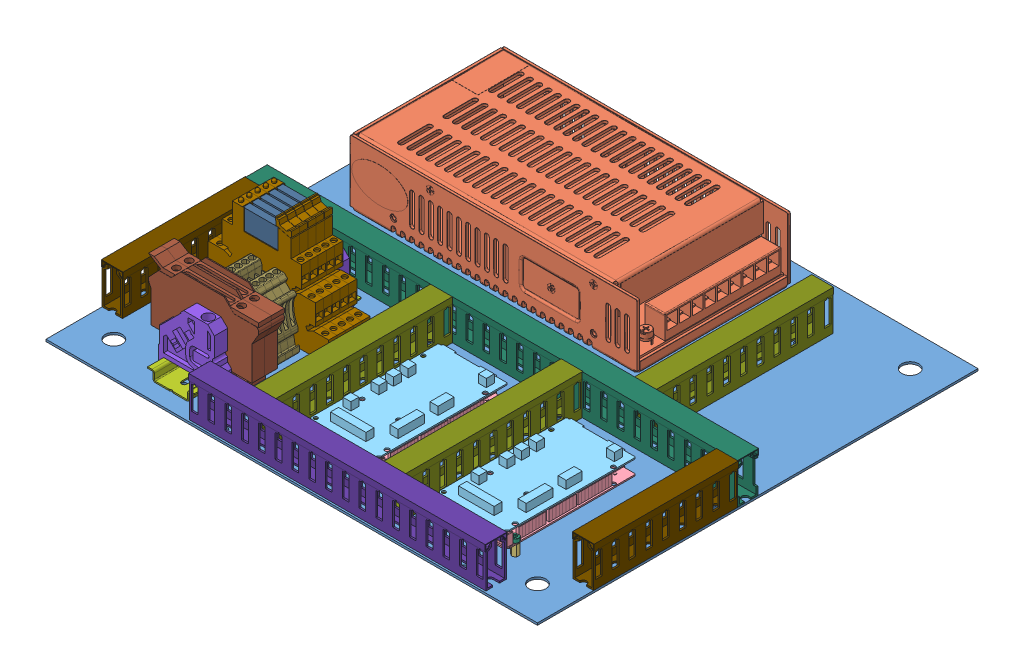
SolidWorks assembly elc component panel, configuration Default. Lengths in mm.
Overall size (369.37 85.56 330.2).
68 component instances, 18 part files, 51 mates.
Components (placement in the parent):
- elc plate-1: elc plate [Default] at (226.2293 207.4053 266.8793) size (368.3 1.59 330.2)
- power supply with standoffs-1: power supply with standoffs [Default] at (35.6304 133.9192 294.786) x (0 0 -1) z (1 0 0) size (115.2 58.27 215)
  - __-1: __ [По умолчанию] at (110.1067 83.0736 152.0488) size (115.2 50.11 215)
  - 95783A055_NYLON 6 6 MALE-FEMALE THREADED HEX STANDOFF-1: 95783A055_NYLON 6 6 MALE-FEMALE THREADED HEX STANDOFF [95783A055] at (85.1067 81.4236 77.0488) x (0 1 0) z (0 0 1) size (13.03 5.2 4.5)
  - 95783A055_NYLON 6 6 MALE-FEMALE THREADED HEX STANDOFF-2: 95783A055_NYLON 6 6 MALE-FEMALE THREADED HEX STANDOFF [95783A055] at (135.1067 81.4236 77.0488) x (0 1 0) z (-0.939028 0 -0.343839) size (13.03 5.2 4.5)
  - 95783A055_NYLON 6 6 MALE-FEMALE THREADED HEX STANDOFF-3: 95783A055_NYLON 6 6 MALE-FEMALE THREADED HEX STANDOFF [95783A055] at (135.1067 81.4236 227.0488) x (0 1 0) z (-0.996262 0 -0.086381) size (13.03 5.2 4.5)
  - 95783A055_NYLON 6 6 MALE-FEMALE THREADED HEX STANDOFF-4: 95783A055_NYLON 6 6 MALE-FEMALE THREADED HEX STANDOFF [95783A055] at (85.1067 81.4236 227.0488) x (0 1 0) z (-0.990494 0 -0.137554) size (13.03 5.2 4.5)
- arduino board assembly-1: arduino board assembly [Default] at (260.6228 173.6976 405.5467) x (0 0 -1) z (1 0 0) size (100 30.86 52.88)
  - ArduinoMega2560 CORRECTED-1: ArduinoMega2560 CORRECTED [Default] at (48.9673 43.2952 72.715) size (100 11.65 51.63)
  - breakout board-1: breakout board [Default] at (48.9673 54.2952 72.715) size (100 7 51.63)
  - 95783A055_NYLON 6 6 MALE-FEMALE THREADED HEX STANDOFF-1: 95783A055_NYLON 6 6 MALE-FEMALE THREADED HEX STANDOFF [95783A055] at (84.2031 36.9452 49.5995) x (0 -1 0) z (0 0 1) size (13.03 5.2 4.5)
  - 95783A055_NYLON 6 6 MALE-FEMALE THREADED HEX STANDOFF-2: 95783A055_NYLON 6 6 MALE-FEMALE THREADED HEX STANDOFF [95783A055] at (3.483 36.9452 49.7272) x (0 -1 0) z (0 0 1) size (13.03 5.2 4.5)
  - 95783A055_NYLON 6 6 MALE-FEMALE THREADED HEX STANDOFF-3: 95783A055_NYLON 6 6 MALE-FEMALE THREADED HEX STANDOFF [95783A055] at (9.6911 36.9452 96.9805) x (0 -1 0) z (0 0 1) size (13.03 5.2 4.5)
  - 91290A110_BLACK-OXIDE CLASS 12.9 SOCKET HEAD CAP SCREW-1: 91290A110_BLACK-OXIDE CLASS 12.9 SOCKET HEAD CAP SCREW [91290A110] at (9.6911 39.2952 96.9805) x (1 0 0) z (0 -1 0) size (5.5 5.5 8.18)
  - 91290A110_BLACK-OXIDE CLASS 12.9 SOCKET HEAD CAP SCREW-2: 91290A110_BLACK-OXIDE CLASS 12.9 SOCKET HEAD CAP SCREW [91290A110] at (84.2031 39.2952 49.5995) x (1 0 0) z (0 -1 0) size (5.5 5.5 8.18)
  - 91290A110_BLACK-OXIDE CLASS 12.9 SOCKET HEAD CAP SCREW-3: 91290A110_BLACK-OXIDE CLASS 12.9 SOCKET HEAD CAP SCREW [91290A110] at (3.483 39.2952 49.7272) x (1 0 0) z (0 -1 0) size (5.5 5.5 8.18)
- din rail assmbly-1: din rail assmbly [Default] at (226.6874 101.8607 473.572) x (-1 0 0) z (0 0 -1) size (90.31 80.69 125)
  - DIN 59_0-1: DIN 59_0 [00] at (103.6081 107.1321 54.2926) size (35 7.5 125)
  - SEIMENS 8WA1 808 DIN RAIL END RETAINER-1: SEIMENS 8WA1 808 DIN RAIL END RETAINER [Default] at (102.6081 107.6321 71.2884) size (45 44.95 10)
  - SEIMENS 8WA1 808 DIN RAIL END RETAINER-3: SEIMENS 8WA1 808 DIN RAIL END RETAINER [Default] at (102.6081 107.6321 162.4924) size (45 44.95 10)
  - 3812830-8: 3812830 [Default] at (102.7638 140.3713 56.6988) x (0 0 -1) z (1 0 0) size (6.2 76.69 90.31)
    - 3812830A-1: 3812830A [Default] at (-75.9936 -29.2392 18.3443) size (6.2 76.69 90.31)
    - 3812830B-1: 3812830B [Default] at (-75.3936 25.9608 19.6) size (5 19.3 28)
  - 3812830-9: 3812830 [Default] at (102.7638 140.3713 62.8988) x (0 0 -1) z (1 0 0) size (6.2 76.69 90.31)
    - 3812830A-1: 3812830A [Default] at (-75.9936 -29.2392 18.3443) size (6.2 76.69 90.31)
    - 3812830B-1: 3812830B [Default] at (-75.3936 25.9608 19.6) size (5 19.3 28)
  - 3812830-10: 3812830 [Default] at (102.7638 140.3713 69.0988) x (0 0 -1) z (1 0 0) size (6.2 76.69 90.31)
    - 3812830A-1: 3812830A [Default] at (-75.9936 -29.2392 18.3443) size (6.2 76.69 90.31)
    - 3812830B-1: 3812830B [Default] at (-75.3936 25.9608 19.6) size (5 19.3 28)
  - 3812830-11: 3812830 [Default] at (102.7638 140.3713 75.2988) x (0 0 -1) z (1 0 0) size (6.2 76.69 90.31)
    - 3812830A-1: 3812830A [Default] at (-75.9936 -29.2392 18.3443) size (6.2 76.69 90.31)
    - 3812830B-1: 3812830B [Default] at (-75.3936 25.9608 19.6) size (5 19.3 28)
  - 3812830-12: 3812830 [Default] at (102.7638 140.3713 81.4988) x (0 0 -1) z (1 0 0) size (6.2 76.69 90.31)
    - 3812830A-1: 3812830A [Default] at (-75.9936 -29.2392 18.3443) size (6.2 76.69 90.31)
    - 3812830B-1: 3812830B [Default] at (-75.3936 25.9608 19.6) size (5 19.3 28)
  - Din fuse-1: Din fuse [Default] at (59.9389 109.5521 90.7664) size (82.55 57.15 9.65)
  - Din fuse-2: Din fuse [Default] at (59.9389 109.5521 81.1144) size (82.55 57.15 9.65)
  - dinrail_Terminal-11: dinrail_Terminal [Default] at (121.1081 114.6321 95.5924) size (48 46.85 5.15)
  - dinrail_Terminal-12: dinrail_Terminal [Default] at (121.1081 114.6321 100.7424) size (48 46.85 5.15)
  - dinrail_Terminal-13: dinrail_Terminal [Default] at (121.1081 114.6321 111.0424) size (48 46.85 5.15)
  - dinrail_Terminal-16: dinrail_Terminal [Default] at (121.1081 114.6321 105.8924) size (48 46.85 5.15)
  - dinrail_Terminal-17: dinrail_Terminal [Default] at (121.1081 114.6321 116.1924) size (48 46.85 5.15)
  - dinrail_Terminal-18: dinrail_Terminal [Default] at (121.1081 114.6321 121.3424) size (48 46.85 5.15)
- arduino board assembly-2: arduino board assembly [Default] at (164.5922 173.6976 405.5467) x (0 0 -1) z (1 0 0) size (100 30.86 52.88)
  - ArduinoMega2560 CORRECTED-1: ArduinoMega2560 CORRECTED [Default] at (48.9673 43.2952 72.715) size (100 11.65 51.63)
  - breakout board-1: breakout board [Default] at (48.9673 54.2952 72.715) size (100 7 51.63)
  - 95783A055_NYLON 6 6 MALE-FEMALE THREADED HEX STANDOFF-1: 95783A055_NYLON 6 6 MALE-FEMALE THREADED HEX STANDOFF [95783A055] at (84.2031 36.9452 49.5995) x (0 -1 0) z (0 0 1) size (13.03 5.2 4.5)
  - 95783A055_NYLON 6 6 MALE-FEMALE THREADED HEX STANDOFF-2: 95783A055_NYLON 6 6 MALE-FEMALE THREADED HEX STANDOFF [95783A055] at (3.483 36.9452 49.7272) x (0 -1 0) z (0 0 1) size (13.03 5.2 4.5)
  - 95783A055_NYLON 6 6 MALE-FEMALE THREADED HEX STANDOFF-3: 95783A055_NYLON 6 6 MALE-FEMALE THREADED HEX STANDOFF [95783A055] at (9.6911 36.9452 96.9805) x (0 -1 0) z (0 0 1) size (13.03 5.2 4.5)
  - 91290A110_BLACK-OXIDE CLASS 12.9 SOCKET HEAD CAP SCREW-1: 91290A110_BLACK-OXIDE CLASS 12.9 SOCKET HEAD CAP SCREW [91290A110] at (9.6911 39.2952 96.9805) x (1 0 0) z (0 -1 0) size (5.5 5.5 8.18)
  - 91290A110_BLACK-OXIDE CLASS 12.9 SOCKET HEAD CAP SCREW-2: 91290A110_BLACK-OXIDE CLASS 12.9 SOCKET HEAD CAP SCREW [91290A110] at (84.2031 39.2952 49.5995) x (1 0 0) z (0 -1 0) size (5.5 5.5 8.18)
  - 91290A110_BLACK-OXIDE CLASS 12.9 SOCKET HEAD CAP SCREW-3: 91290A110_BLACK-OXIDE CLASS 12.9 SOCKET HEAD CAP SCREW [91290A110] at (3.483 39.2952 49.7272) x (1 0 0) z (0 -1 0) size (5.5 5.5 8.18)
- 92497A200_ZINC YELLOW-CHROMATE PLATED STEEL HEX NUT-1: 92497A200_ZINC YELLOW-CHROMATE PLATED STEEL HEX NUT [92497A200] at (214.3194 206.2053 402.0637) x (1 0 0) z (0 1 0) size (5.5 6.35 2.78)
- 92497A200_ZINC YELLOW-CHROMATE PLATED STEEL HEX NUT-2: 92497A200_ZINC YELLOW-CHROMATE PLATED STEEL HEX NUT [92497A200] at (214.1917 206.2053 321.3436) x (1 0 0) z (0 1 0) size (5.5 6.35 2.78)
- 92497A200_ZINC YELLOW-CHROMATE PLATED STEEL HEX NUT-3: 92497A200_ZINC YELLOW-CHROMATE PLATED STEEL HEX NUT [92497A200] at (261.5727 206.2053 395.8556) x (1 0 0) z (0 1 0) size (5.5 6.35 2.78)
- 92497A200_ZINC YELLOW-CHROMATE PLATED STEEL HEX NUT-4: 92497A200_ZINC YELLOW-CHROMATE PLATED STEEL HEX NUT [92497A200] at (310.3501 206.2053 402.0637) x (1 0 0) z (0 1 0) size (5.5 6.35 2.78)
- 92497A200_ZINC YELLOW-CHROMATE PLATED STEEL HEX NUT-5: 92497A200_ZINC YELLOW-CHROMATE PLATED STEEL HEX NUT [92497A200] at (310.2224 206.2053 321.3436) x (1 0 0) z (0 1 0) size (5.5 6.35 2.78)
- 92497A200_ZINC YELLOW-CHROMATE PLATED STEEL HEX NUT-6: 92497A200_ZINC YELLOW-CHROMATE PLATED STEEL HEX NUT [92497A200] at (357.6034 206.2053 395.8556) x (1 0 0) z (0 1 0) size (5.5 6.35 2.78)
- 92095A177_18-8 SS BUTTON-HEAD SOCKET CAP SCREW-1: 92095A177_18-8 SS BUTTON-HEAD SOCKET CAP SCREW [92095A177] at (262.6793 205.7553 159.6793) x (1 0 0) z (0 -1 0) size (5.7 5.7 6.94)
- 92095A177_18-8 SS BUTTON-HEAD SOCKET CAP SCREW-3: 92095A177_18-8 SS BUTTON-HEAD SOCKET CAP SCREW [92095A177] at (112.6793 205.7553 159.6793) x (1 0 0) z (0 -1 0) size (5.7 5.7 6.94)
- 92095A177_18-8 SS BUTTON-HEAD SOCKET CAP SCREW-4: 92095A177_18-8 SS BUTTON-HEAD SOCKET CAP SCREW [92095A177] at (112.6793 205.7553 209.6793) x (1 0 0) z (0 -1 0) size (5.7 5.7 6.94)
- small panduit 1-2: small panduit 1 [Default] at (435.7793 210.2628 274.3593) size (368.3 30.38 16.31)
- small panduit 4-6: small panduit 4 [Default] at (286.3538 210.2628 21.6293) x (0 0 -1) z (1 0 0) size (133.35 30.38 16.31)
- small panduit 4-7: small panduit 4 [Default] at (188.9955 210.2628 21.6293) x (0 0 -1) z (1 0 0) size (133.35 30.38 16.31)
- small panduit 4-8: small panduit 4 [Default] at (325.6017 210.2628 527.0893) x (0 0 1) z (-1 0 0) size (133.35 30.38 16.31)
- small panduit 3-2: small panduit 3 [Default] at (541.8293 210.2628 422.9493) size (222.25 30.38 16.31)
- small panduit 2-10: small panduit 2 [Default] at (49.6993 210.2628 -3.7707) x (0 0 -1) z (1 0 0) size (107.95 30.38 16.31)
- small panduit 2-11: small panduit 2 [Default] at (402.7593 210.2628 -3.7707) x (0 0 -1) z (1 0 0) size (107.95 30.38 16.31)
Mates (geometry in assembly coordinates):
- Coincident4: coincident: plane of elc plate-1 through (226.2293 208.9928 266.8793) normal (0 1 0); plane of arduino board assembly-1/95783A055_NYLON 6 6 MALE-FEMALE THREADED HEX STANDOFF-1 through (310.2224 208.9928 318.7455) normal (0 -1 0)
- Coincident5: coincident: plane of elc plate-1 through (226.2293 208.9928 266.8793) normal (0 1 0); plane of din rail assmbly-1/DIN 59_0-1 through (136.5793 208.9928 294.2793) normal (0 -1 0)
- Parallel2: parallel: plane of elc plate-1 through (410.3793 208.9928 101.7793) normal (1 0 0); plane of arduino board assembly-1/ArduinoMega2560 CORRECTED-1 through (359.5793 207.9928 308.1039) normal (1 0 0)
- Coincident8: coincident: plane of elc plate-1 through (226.2293 208.9928 266.8793) normal (0 1 0); plane of arduino board assembly-2/95783A055_NYLON 6 6 MALE-FEMALE THREADED HEX STANDOFF-3 through (261.5727 208.9928 393.2575) normal (0 -1 0)
- Parallel3: parallel: plane of arduino board assembly-1/breakout board-1 through (307.9466 218.9928 306.5793) normal (-1 0 0); line of arduino board assembly-2/ArduinoMega2560 CORRECTED-1 through (263.5486 216.9928 308.1039) axis (0 0 1)
- Coincident28: coincident: plane of arduino board assembly-1/ArduinoMega2560 CORRECTED-1 through (350.3515 225.9928 306.5793) normal (0 0 -1); line of arduino board assembly-2/ArduinoMega2560 CORRECTED-1 through (242.4708 225.9928 306.5793) axis (1 0 0)
- Coincident36: coincident: plane of elc plate-1 through (226.2293 207.4053 266.8793) normal (0 -1 0); plane of 92497A200_ZINC YELLOW-CHROMATE PLATED STEEL HEX NUT-1 through (211.5694 207.4053 400.476) normal (0 1 0)
- Concentric1: concentric: cylinder of arduino board assembly-2/91290A110_BLACK-OXIDE CLASS 12.9 SOCKET HEAD CAP SCREW-3 through (214.3194 220.9928 402.0637) axis (0 -1 0) radius 2.75; circle of 92497A200_ZINC YELLOW-CHROMATE PLATED STEEL HEX NUT-1
- Coincident37: coincident: plane of elc plate-1 through (226.2293 207.4053 266.8793) normal (0 -1 0); plane of 92497A200_ZINC YELLOW-CHROMATE PLATED STEEL HEX NUT-3 through (258.8227 207.4053 394.2679) normal (0 1 0)
- Concentric2: concentric: cylinder of arduino board assembly-2/91290A110_BLACK-OXIDE CLASS 12.9 SOCKET HEAD CAP SCREW-1 through (261.5727 220.9928 395.8556) axis (0 -1 0) radius 2.75; circle of 92497A200_ZINC YELLOW-CHROMATE PLATED STEEL HEX NUT-3
- Coincident38: coincident: plane of elc plate-1 through (226.2293 207.4053 266.8793) normal (0 -1 0); plane of 92497A200_ZINC YELLOW-CHROMATE PLATED STEEL HEX NUT-2 through (211.4417 207.4053 319.7559) normal (0 1 0)
- Concentric3: concentric: cylinder of elc plate-1 through (214.1917 208.9938 321.3436) axis (0 -1 0) radius 1.665; circle of 92497A200_ZINC YELLOW-CHROMATE PLATED STEEL HEX NUT-2
- Coincident39: coincident: plane of elc plate-1 through (226.2293 207.4053 266.8793) normal (0 -1 0); plane of 92497A200_ZINC YELLOW-CHROMATE PLATED STEEL HEX NUT-4 through (307.6001 207.4053 400.476) normal (0 1 0)
- Concentric4: concentric: cylinder of elc plate-1 through (310.3501 208.9938 402.0637) axis (0 -1 0) radius 1.665; circle of 92497A200_ZINC YELLOW-CHROMATE PLATED STEEL HEX NUT-4
- Coincident40: coincident: plane of elc plate-1 through (226.2293 207.4053 266.8793) normal (0 -1 0); plane of 92497A200_ZINC YELLOW-CHROMATE PLATED STEEL HEX NUT-6 through (354.8534 207.4053 394.2679) normal (0 1 0)
- Concentric5: concentric: cylinder of elc plate-1 through (357.6034 208.9938 395.8556) axis (0 -1 0) radius 1.665; circle of 92497A200_ZINC YELLOW-CHROMATE PLATED STEEL HEX NUT-6
- Coincident41: coincident: plane of elc plate-1 through (226.2293 207.4053 266.8793) normal (0 -1 0); plane of 92497A200_ZINC YELLOW-CHROMATE PLATED STEEL HEX NUT-5 through (307.4724 207.4053 319.7559) normal (0 1 0)
- Concentric6: concentric: cylinder of elc plate-1 through (310.2224 208.9938 321.3436) axis (0 -1 0) radius 1.665; circle of 92497A200_ZINC YELLOW-CHROMATE PLATED STEEL HEX NUT-5
- Coincident43: coincident: plane of elc plate-1 through (226.2293 207.4053 266.8793) normal (0 -1 0); plane of 92095A177_18-8 SS BUTTON-HEAD SOCKET CAP SCREW-1 through (262.6793 207.4053 156.8293) normal (0 1 0)
- Concentric8: concentric: cylinder of elc plate-1 through (262.6793 207.4043 159.6793) axis (0 1 0) radius 1.665; cylinder of 92095A177_18-8 SS BUTTON-HEAD SOCKET CAP SCREW-1 through (262.6793 205.7553 159.6793) axis (0 -1 0) radius 2.85
- Coincident44: coincident: plane of elc plate-1 through (226.2293 207.4053 266.8793) normal (0 -1 0); plane of 92095A177_18-8 SS BUTTON-HEAD SOCKET CAP SCREW-4 through (112.6793 207.4053 206.8293) normal (0 1 0)
- Concentric9: concentric: cylinder of elc plate-1 through (112.6793 207.4043 209.6793) axis (0 1 0) radius 1.665; cylinder of 92095A177_18-8 SS BUTTON-HEAD SOCKET CAP SCREW-4 through (112.6793 205.7553 209.6793) axis (0 -1 0) radius 2.85
- Coincident45: coincident: plane of elc plate-1 through (226.2293 207.4053 266.8793) normal (0 -1 0); plane of 92095A177_18-8 SS BUTTON-HEAD SOCKET CAP SCREW-3 through (112.6793 207.4053 156.8293) normal (0 1 0)
- Concentric10: concentric: cylinder of elc plate-1 through (112.6793 207.4043 159.6793) axis (0 1 0) radius 1.665; cylinder of 92095A177_18-8 SS BUTTON-HEAD SOCKET CAP SCREW-3 through (112.6793 205.7553 159.6793) axis (0 -1 0) radius 2.85
- Coincident62: coincident: plane of elc plate-1 through (226.2293 208.9928 266.8793) normal (0 1 0); plane of power supply with standoffs-1/95783A055_NYLON 6 6 MALE-FEMALE THREADED HEX STANDOFF-1 through (112.6793 208.9928 212.2774) normal (0 -1 0)
- Distance1: distance = 38.1 mm: plane of power supply with standoffs-1/__-1 through (80.1793 265.9928 184.6793) normal (-1 0 0); plane of elc plate-1 through (42.0793 208.9928 101.7793) normal (-1 0 0)
- Distance2: distance = 25.4 mm: plane of power supply with standoffs-1/__-1 through (80.1793 218.9928 127.1793) normal (0 0 -1); plane of elc plate-1 through (42.0793 208.9928 101.7793) normal (0 0 -1)
- Parallel4: parallel: line of elc plate-1 through (410.3793 207.4053 101.7793) axis (-1 0 0); plane of din rail assmbly-1/DIN 59_0-1 through (109.5793 209.9928 294.2793) normal (0 0 -1)
- Distance3: distance = 50.8 mm: plane of arduino board assembly-1/ArduinoMega2560 CORRECTED-1 through (359.5793 207.9928 308.1039) normal (1 0 0); plane of elc plate-1 through (410.3793 208.9928 101.7793) normal (1 0 0)
- Parallel5: parallel: plane of din rail assmbly-1/DIN 59_0-1 through (109.5793 216.4928 419.2793) normal (0 0 1); plane of arduino board assembly-2/ArduinoMega2560 CORRECTED-1 through (263.8072 217.9928 406.5793) normal (0 0 1)
- Distance4: distance = 12.7 mm: plane of din rail assmbly-1/DIN 59_0-1 through (136.5793 216.4928 419.2793) normal (0 0 1); plane of elc plate-1 through (42.0793 208.9928 431.9793) normal (0 0 1)
- Distance5: distance = 63.5 mm: plane of din rail assmbly-1/DIN 59_0-1 through (105.5793 216.4928 419.2793) normal (-1 0 0); plane of elc plate-1 through (42.0793 208.9928 101.7793) normal (-1 0 0)
- Distance6: distance = 25.4 mm: plane of arduino board assembly-1/ArduinoMega2560 CORRECTED-1 through (359.8379 217.9928 406.5793) normal (0 0 1); plane of elc plate-1 through (42.0793 208.9928 431.9793) normal (0 0 1)
- Coincident71: coincident: plane of elc plate-1 through (226.2293 208.9928 266.8793) normal (0 1 0); plane of small panduit 1-2 through (829.4793 208.9928 274.3593) normal (0 -1 0)
- Coincident72: coincident: plane of elc plate-1 through (410.3793 208.9928 101.7793) normal (1 0 0); plane of small panduit 1-2 through (410.3793 208.9928 266.2059) normal (1 0 0)
- Coincident73: coincident: plane of elc plate-1 through (226.2293 208.9928 266.8793) normal (0 1 0); plane of small panduit 4-6 through (286.3538 208.9928 -372.0707) normal (0 -1 0)
- Coincident74: coincident: plane of small panduit 1-2 through (829.4793 208.9928 281.9793) normal (0 0 1); plane of small panduit 4-6 through (278.2004 208.9928 281.9793) normal (0 0 -1)
- Distance7: distance = 150 mm: plane of small panduit 1-2 through (829.4793 208.9928 281.9793) normal (0 0 1); line of elc plate-1 through (42.0793 207.4053 431.9793) axis (1 0 0)
- Coincident76: coincident: plane of small panduit 1-2 through (829.4793 208.9928 281.9793) normal (0 0 1); plane of small panduit 4-7 through (180.8421 208.9928 281.9793) normal (0 0 -1)
- Coincident77: coincident: plane of elc plate-1 through (226.2293 208.9928 266.8793) normal (0 1 0); plane of small panduit 4-7 through (188.9955 208.9928 -372.0707) normal (0 -1 0)
- Coincident78: coincident: plane of small panduit 1-2 through (829.4793 208.9928 266.7393) normal (0 0 -1); plane of small panduit 4-8 through (333.7551 208.9928 266.7393) normal (0 0 1)
- Coincident79: coincident: plane of elc plate-1 through (226.2293 208.9928 266.8793) normal (0 1 0); plane of small panduit 4-8 through (325.6017 208.9928 920.7893) normal (0 -1 0)
- Coincident80: coincident: plane of elc plate-1 through (226.2293 208.9928 266.8793) normal (0 1 0); plane of small panduit 3-2 through (935.5293 208.9928 422.9493) normal (0 -1 0)
- Coincident81: coincident: plane of small panduit 4-6 through (286.3538 210.2628 415.3293) normal (0 0 1); plane of small panduit 3-2 through (935.5293 208.9928 415.3293) normal (0 0 -1)
- Distance8: distance = 40 mm: plane of small panduit 3-2 through (370.3793 208.9928 414.7959) normal (1 0 0); plane of elc plate-1 through (410.3793 208.9928 101.7793) normal (1 0 0)
- Coincident83: coincident: plane of small panduit 1-2 through (829.4793 208.9928 281.9793) normal (0 0 1); plane of small panduit 2-10 through (41.5459 208.9928 281.9793) normal (0 0 -1)
- Coincident84: coincident: plane of elc plate-1 through (226.2293 208.9928 266.8793) normal (0 1 0); plane of small panduit 2-10 through (49.6993 208.9928 -397.4707) normal (0 -1 0)
- Coincident85: coincident: plane of elc plate-1 through (42.0793 208.9928 101.7793) normal (-1 0 0); plane of small panduit 2-10 through (42.0793 208.9928 -397.4707) normal (-1 0 0)
- Coincident86: coincident: plane of small panduit 1-2 through (829.4793 208.9928 281.9793) normal (0 0 1); plane of small panduit 2-11 through (394.6059 208.9928 281.9793) normal (0 0 -1)
- Coincident87: coincident: plane of elc plate-1 through (226.2293 208.9928 266.8793) normal (0 1 0); plane of small panduit 2-11 through (402.7593 208.9928 -397.4707) normal (0 -1 0)
- Coincident88: coincident: line of elc plate-1 through (410.3793 207.4053 431.9793) axis (0 0 -1); plane of small panduit 2-11 through (410.3793 208.9928 -397.4707) normal (1 0 0)
